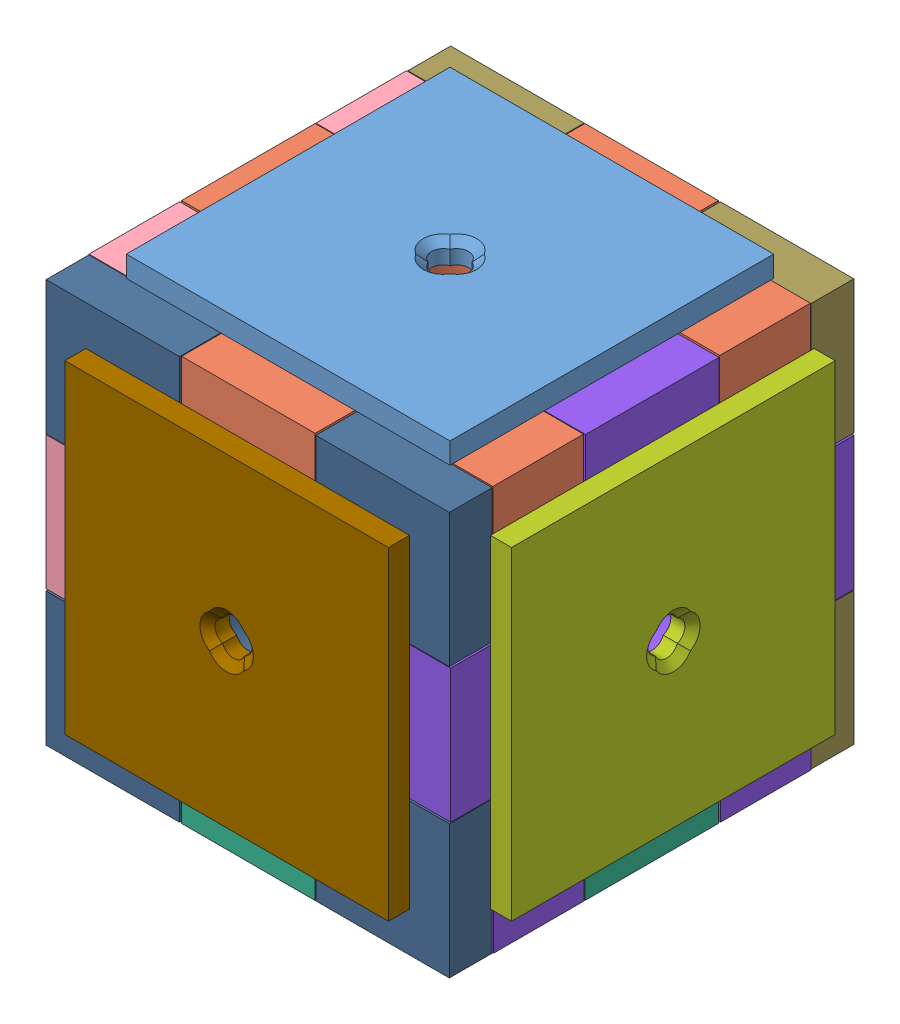
SolidWorks assembly cube_12, configuration cube12. Lengths in mm.
Overall size (33.65 33.65 33.65).
12 component instances, 12 part files, 6 mates.
Components (placement in the parent):
- panel_R^cube_12-13: panel_R^cube_12 [cube01] x (-1 0 0) z (0 0 1) size (24.38 1.59 24.38) (virtual)
- acrylic_R^cube_12-1: acrylic_R^cube_12 [A] at origin size (30.38 3.23 30.38) (virtual)
- panel_O^cube_12-8: panel_O^cube_12 [cube01] x (0 -1 0) z (0 0 1) size (24.38 1.59 24.38) (virtual)
- acrylic_O^cube_12-23: acrylic_O^cube_12 [A] x (0 1 0) z (0 0 1) size (30.38 3.23 30.38) (virtual)
- panel_Y^cube_12-9: panel_Y^cube_12 [cube01] at origin size (24.38 1.59 24.38) (virtual)
- acrylic_Y^cube_12-24: acrylic_Y^cube_12 [A] x (-1 0 0) z (0 0 1) size (30.38 3.23 30.38) (virtual)
- panel_G^cube_12-10: panel_G^cube_12 [cube01] x (0 1 0) z (0 0 1) size (24.38 1.59 24.38) (virtual)
- acrylic_G^cube_12-25: acrylic_G^cube_12 [A] x (0 -1 0) z (0 0 1) size (30.38 3.23 30.38) (virtual)
- panel_C^cube_12-11: panel_C^cube_12 [cube01] x (-1 0 0) z (0 -1 0) size (24.38 1.59 24.38) (virtual)
- acrylic_C^cube_12-26: acrylic_C^cube_12 [B] x (1 0 0) z (0 -1 0) size (30.38 3.23 30.38) (virtual)
- panel_B^cube_12-13: panel_B^cube_12 [cube01] x (-1 0 0) z (0 1 0) size (24.38 1.59 24.38) (virtual)
- acrylic_B^cube_12-27: acrylic_B^cube_12 [B] x (1 0 0) z (0 1 0) size (30.38 3.23 30.38) (virtual)
Mates (geometry in assembly coordinates):
- Coincident1: coincident aligned: plane of panel_R^cube_12-13 through (0 0 0) normal (0 0 1); plane of assembly through (0 0 0) normal (0 0 1)
- Coincident2: coincident anti-aligned: plane of panel_R^cube_12-13; plane of assembly through (0 0 0) normal (1 0 0)
- Coincident3: coincident anti-aligned: plane of panel_R^cube_12-13; plane of assembly through (0 0 0) normal (0 1 0)
- Coincident4: coincident aligned: plane of acrylic_R^cube_12-1 through (0 0 0) normal (0 0 1); plane of assembly through (0 0 0) normal (0 0 1)
- Coincident5: coincident aligned: plane of acrylic_R^cube_12-1 through (0 0 0) normal (1 0 0); plane of assembly through (0 0 0) normal (1 0 0)
- Coincident6: coincident aligned: plane of ? through (0 0 0) normal (0 1 0); plane of assembly through (0 0 0) normal (0 1 0)
